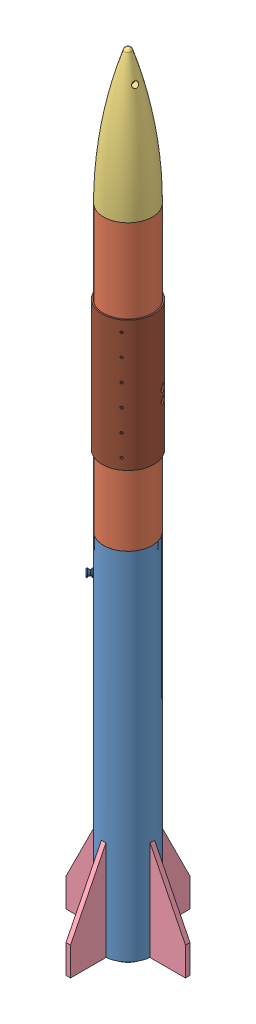
SolidWorks assembly ASSY_ROCKET_MASTER, configuration Default. Lengths in mm.
Overall size (168 1100 168).
745 component instances, 461 part files, 40 mates.
Components (placement in the parent):
- ROCKET_BODY_TUBE_LOWER-1: ROCKET_BODY_TUBE_LOWER [Default] at origin size (68.5 500 68.5)
- ROCKET_BODY_TUBE_UPPER-1: ROCKET_BODY_TUBE_UPPER [Default] at (0 500 0) x (0 0 1) z (-1 0 0) size (68.5 400 68.5)
- ROCKET_NOSE_CONE-1: ROCKET_NOSE_CONE [Default] at (0 840 0) x (0.965412 0 0.260729) z (-0.260729 0 0.965412) size (68.5 250 68.5)
- ROCKET_FIN_LOWER-1: ROCKET_FIN_LOWER [Default] at origin size (6.35 140 63)
- ROCKET_FIN_LOWER-2: ROCKET_FIN_LOWER [Default] x (0 0 1) z (-1 0 0) size (6.35 140 63)
- ROCKET_FIN_LOWER-3: ROCKET_FIN_LOWER [Default] x (-1 0 0) z (0 0 -1) size (6.35 140 63)
- ROCKET_FIN_LOWER-4: ROCKET_FIN_LOWER [Default] x (0 0 -1) z (1 0 0) size (6.35 140 63)
- ROCKET_BODY_COUPLER-1: ROCKET_BODY_COUPLER [Default] at (0 437.6 0) size (64.9 152.4 64.9)
- ASSY_HYDRA_MASTER-1: ASSY_HYDRA_MASTER [Default] at (0 713.5 0) x (0.707107 0 0.707107) z (0 1 0) size (64 66.9 228.49)
  - HYDRA_V4_NAV-1: HYDRA_V4_NAV [Default] at origin size (50 44 11.77)
    - Open CASCADE STEP translator 7.5 734-1: Open CASCADE STEP translator 7.5 734 [Default] at origin size (50 44 1.75)
    - Open CASCADE STEP translator 7.5 766-1: Open CASCADE STEP translator 7.5 766 [Default] at origin size (2.53 3.23 1.01)
    - Open CASCADE STEP translator 7.5 767-1: Open CASCADE STEP translator 7.5 767 [Default] at origin size (2.5 3.2 0)
    - Open CASCADE STEP translator 7.5 769-1: Open CASCADE STEP translator 7.5 769 [Default] at origin size (0.26 1.24 0)
    - Open CASCADE STEP translator 7.5 770-1: Open CASCADE STEP translator 7.5 770 [Default] at origin size (2.9 1.6 1.31)
    - Open CASCADE STEP translator 7.5 771-1: Open CASCADE STEP translator 7.5 771 [Default] at origin size (0.3 0.6 0.86)
    - Open CASCADE STEP translator 7.5 772-1: Open CASCADE STEP translator 7.5 772 [Default] at origin size (0.3 0.6 0.86)
    - Open CASCADE STEP translator 7.5 773-1: Open CASCADE STEP translator 7.5 773 [Default] at origin size (0.3 0.6 0.86)
    - Open CASCADE STEP translator 7.5 774-1: Open CASCADE STEP translator 7.5 774 [Default] at origin size (0.3 0.6 0.86)
    - Open CASCADE STEP translator 7.5 775-1: Open CASCADE STEP translator 7.5 775 [Default] at origin size (0.4 0.4 0.01)
    - Open CASCADE STEP translator 7.5 776-1: Open CASCADE STEP translator 7.5 776 [Default] at origin size (0.29 1.22 0.01)
    - Open CASCADE STEP translator 7.5 777-1: Open CASCADE STEP translator 7.5 777 [Default] at origin size (0.3 0.6 0.86)
    - Open CASCADE STEP translator 7.5 778-1: Open CASCADE STEP translator 7.5 778 [Default] at origin size (0.3 0.6 0.86)
    - Open CASCADE STEP translator 7.5 779-1: Open CASCADE STEP translator 7.5 779 [Default] at origin size (0.3 0.6 0.86)
    - Open CASCADE STEP translator 7.5 780-1: Open CASCADE STEP translator 7.5 780 [Default] at origin size (0.3 0.6 0.86)
    - Open CASCADE STEP translator 7.5 781-1: Open CASCADE STEP translator 7.5 781 [Default] at origin size (3.25 2.93 1.32)
    - Open CASCADE STEP translator 7.5 782-1: Open CASCADE STEP translator 7.5 782 [Default] at origin size (0.59 0.66 0.86)
    - Open CASCADE STEP translator 7.5 783-1: Open CASCADE STEP translator 7.5 783 [Default] at origin size (0.59 0.66 0.86)
    - Open CASCADE STEP translator 7.5 784-1: Open CASCADE STEP translator 7.5 784 [Default] at origin size (0.59 0.66 0.86)
    - Open CASCADE STEP translator 7.5 785-1: Open CASCADE STEP translator 7.5 785 [Default] at origin size (0.59 0.66 0.86)
    - Open CASCADE STEP translator 7.5 786-1: Open CASCADE STEP translator 7.5 786 [Default] at origin size (0.4 0.4 0.01)
    - Open CASCADE STEP translator 7.5 787-1: Open CASCADE STEP translator 7.5 787 [Default] at origin size (0.65 1.09 0.01)
    - Open CASCADE STEP translator 7.5 788-1: Open CASCADE STEP translator 7.5 788 [Default] at origin size (0.59 0.66 0.86)
    - Open CASCADE STEP translator 7.5 789-1: Open CASCADE STEP translator 7.5 789 [Default] at origin size (0.59 0.66 0.86)
    - Open CASCADE STEP translator 7.5 790-1: Open CASCADE STEP translator 7.5 790 [Default] at origin size (0.59 0.66 0.86)
    - Open CASCADE STEP translator 7.5 791-1: Open CASCADE STEP translator 7.5 791 [Default] at origin size (0.59 0.66 0.86)
    - Open CASCADE STEP translator 7.5 833-1: Open CASCADE STEP translator 7.5 833 [Default] at origin size (0.2 2.2 2.05)
    - Open CASCADE STEP translator 7.5 834-1: Open CASCADE STEP translator 7.5 834 [Default] at origin size (0.2 2.2 2.05)
    - Open CASCADE STEP translator 7.5 835-1: Open CASCADE STEP translator 7.5 835 [Default] at origin size (1.45 1.3 1.05)
    - Open CASCADE STEP translator 7.5 836-1: Open CASCADE STEP translator 7.5 836 [Default] at origin size (5.75 4.05 4.25)
    - Open CASCADE STEP translator 7.5 837-1: Open CASCADE STEP translator 7.5 837 [Default] at origin size (1.45 2.03 0.46)
    - Open CASCADE STEP translator 7.5 838-1: Open CASCADE STEP translator 7.5 838 [Default] at origin size (4.2 3.06 0.01)
    - Open CASCADE STEP translator 7.5 839-1: Open CASCADE STEP translator 7.5 839 [Default] at origin size (14.1 15.2 1.88)
    - Open CASCADE STEP translator 7.5 863-1: Open CASCADE STEP translator 7.5 863 [Default] at origin size (4.1 4.1 0.98)
    - Open CASCADE STEP translator 7.5 864-1: Open CASCADE STEP translator 7.5 864 [Default] at origin size (4.53 6.4 0.96)
    - Open CASCADE STEP translator 7.5 865-1: Open CASCADE STEP translator 7.5 865 [Default] at origin size (6.2 6.4 0.64)
    - Open CASCADE STEP translator 7.5 866-1: Open CASCADE STEP translator 7.5 866 [Default] at origin size (5.96 5.96 2.39)
    - Open CASCADE STEP translator 7.5 867-1: Open CASCADE STEP translator 7.5 867 [Default] at origin size (4.4 4.4 0.72)
    - Open CASCADE STEP translator 7.5 868-1: Open CASCADE STEP translator 7.5 868 [Default] at origin size (6.1 6 0)
    - Open CASCADE STEP translator 7.5 869-1: Open CASCADE STEP translator 7.5 869 [Default] at origin size (0.75 2.66 0)
    - Open CASCADE STEP translator 7.5 870-1: Open CASCADE STEP translator 7.5 870 [Default] at origin size (3.1 3.1 1)
    - Open CASCADE STEP translator 7.5 871-1: Open CASCADE STEP translator 7.5 871 [Default] at origin size (3 2.5 0.81)
    - Open CASCADE STEP translator 7.5 1038-1: Open CASCADE STEP translator 7.5 1038 [Default] at origin size (1.6 1.5 0.2)
    - Open CASCADE STEP translator 7.5 1039-1: Open CASCADE STEP translator 7.5 1039 [Default] at origin size (1.6 1.4 0.19)
    - Open CASCADE STEP translator 7.5 1040-1: Open CASCADE STEP translator 7.5 1040 [Default] at origin size (1.1 1.5 0.36)
    - Open CASCADE STEP translator 7.5 1113-1: Open CASCADE STEP translator 7.5 1113 [Default] at origin size (4.71 4.67 1.1)
    - Open CASCADE STEP translator 7.5 1118-1: Open CASCADE STEP translator 7.5 1118 [Default] at origin size (1.6 1.5 0.2)
    - Open CASCADE STEP translator 7.5 1119-1: Open CASCADE STEP translator 7.5 1119 [Default] at origin size (1.6 1.4 0.19)
    - Open CASCADE STEP translator 7.5 1120-1: Open CASCADE STEP translator 7.5 1120 [Default] at origin size (1.1 1.5 0.36)
    - Open CASCADE STEP translator 7.5 1124-1: Open CASCADE STEP translator 7.5 1124 [Default] at origin size (10.4 9.7 2.7)
    - Open CASCADE STEP translator 7.5 1125-1: Open CASCADE STEP translator 7.5 1125 [Default] at origin size (5 3 0.3)
    - Open CASCADE STEP translator 7.5 1126-1: Open CASCADE STEP translator 7.5 1126 [Default] at origin size (4.46 2.46 0.7)
    - Open CASCADE STEP translator 7.5 1127-1: Open CASCADE STEP translator 7.5 1127 [Default] at origin size (4.6 4.6 1.15)
    - Open CASCADE STEP translator 7.5 1128-1: Open CASCADE STEP translator 7.5 1128 [Default] at origin size (14 14 1.52)
    - Open CASCADE STEP translator 7.5 1129-1: Open CASCADE STEP translator 7.5 1129 [Default] at origin size (16 12.22 0.95)
    - Open CASCADE STEP translator 7.5 1130-1: Open CASCADE STEP translator 7.5 1130 [Default] at origin size (12.22 16 0.95)
    - Open CASCADE STEP translator 7.5 1131-1: Open CASCADE STEP translator 7.5 1131 [Default] at origin size (12.33 12.46 0.1)
    - Open CASCADE STEP translator 7.5 1132-1: Open CASCADE STEP translator 7.5 1132 [Default] at origin size (1.3 3.5 0.06)
    - Open CASCADE STEP translator 7.5 1133-1: Open CASCADE STEP translator 7.5 1133 [Default] at origin size (2 3 0.57)
    - Open CASCADE STEP translator 7.5 1134-1: Open CASCADE STEP translator 7.5 1134 [Default] at origin size (2.2 3.2 0.32)
    - Open CASCADE STEP translator 7.5 1135-1: Open CASCADE STEP translator 7.5 1135 [Default] at origin size (0.46 0.93 0.01)
    - Open CASCADE STEP translator 7.5 1136-1: Open CASCADE STEP translator 7.5 1136 [Default] at origin size (1.3 3.5 0.06)
    - Open CASCADE STEP translator 7.5 1137-1: Open CASCADE STEP translator 7.5 1137 [Default] at origin size (2 3 0.57)
    - Open CASCADE STEP translator 7.5 1138-1: Open CASCADE STEP translator 7.5 1138 [Default] at origin size (2.2 3.2 0.32)
    - Open CASCADE STEP translator 7.5 1139-1: Open CASCADE STEP translator 7.5 1139 [Default] at origin size (0.46 0.93 0.01)
    - Open CASCADE STEP translator 7.5 1209-1: Open CASCADE STEP translator 7.5 1209 [Default] at origin size (2.6 2.6 0.35)
    - Open CASCADE STEP translator 7.5 1210-1: Open CASCADE STEP translator 7.5 1210 [Default] at origin size (7.98 7.97 5.08)
    - Open CASCADE STEP translator 7.5 1211-1: Open CASCADE STEP translator 7.5 1211 [Default] at origin size (6.65 6.86 1.68)
    - Open CASCADE STEP translator 7.5 1212-1: Open CASCADE STEP translator 7.5 1212 [Default] at origin size (6.1 6.49 5.65)
    - Open CASCADE STEP translator 7.5 1213-1: Open CASCADE STEP translator 7.5 1213 [Default] at origin size (11.95 7.6 2.76)
    - Open CASCADE STEP translator 7.5 1214-1: Open CASCADE STEP translator 7.5 1214 [Default] at origin size (1.9 6.7 2.22)
    - Open CASCADE STEP translator 7.5 1215-1: Open CASCADE STEP translator 7.5 1215 [Default] at origin size (6.4 5 1.77)
    - Open CASCADE STEP translator 7.5 1216-1: Open CASCADE STEP translator 7.5 1216 [Default] at origin size (4.77 4.35 0.13)
    - Open CASCADE STEP translator 7.5 1217-1: Open CASCADE STEP translator 7.5 1217 [Default] at origin size (1.9 6.7 2.22)
    - Open CASCADE STEP translator 7.5 1293-1: Open CASCADE STEP translator 7.5 1293 [Default] at origin size (1.6 1.5 0.2)
    - Open CASCADE STEP translator 7.5 1294-1: Open CASCADE STEP translator 7.5 1294 [Default] at origin size (1.6 1.4 0.19)
    - Open CASCADE STEP translator 7.5 1295-1: Open CASCADE STEP translator 7.5 1295 [Default] at origin size (1.1 1.5 0.36)
    - Open CASCADE STEP translator 7.5 1296-1: Open CASCADE STEP translator 7.5 1296 [Default] at origin size (1.6 1.5 0.2)
    - Open CASCADE STEP translator 7.5 1297-1: Open CASCADE STEP translator 7.5 1297 [Default] at origin size (1.6 1.4 0.19)
    - Open CASCADE STEP translator 7.5 1298-1: Open CASCADE STEP translator 7.5 1298 [Default] at origin size (1.1 1.5 0.36)
    - Open CASCADE STEP translator 7.5 1299-1: Open CASCADE STEP translator 7.5 1299 [Default] at origin size (1.3 3.5 0.06)
    - Open CASCADE STEP translator 7.5 1300-1: Open CASCADE STEP translator 7.5 1300 [Default] at origin size (2 3 0.57)
    - Open CASCADE STEP translator 7.5 1301-1: Open CASCADE STEP translator 7.5 1301 [Default] at origin size (2.2 3.2 0.32)
    - Open CASCADE STEP translator 7.5 1302-1: Open CASCADE STEP translator 7.5 1302 [Default] at origin size (0.46 0.93 0.01)
    - Open CASCADE STEP translator 7.5 1303-1: Open CASCADE STEP translator 7.5 1303 [Default] at origin size (5.72 15.88 6.73)
    - Open CASCADE STEP translator 7.5 1304-1: Open CASCADE STEP translator 7.5 1304 [Default] at origin size (1.78 12.7 4.01)
    - Open CASCADE STEP translator 7.5 1305-1: Open CASCADE STEP translator 7.5 1305 [Default] at origin size (5.84 12.7 0.83)
    - Open CASCADE STEP translator 7.5 1306-1: Open CASCADE STEP translator 7.5 1306 [Default] at origin size (5.72 15.88 6.73)
    - Open CASCADE STEP translator 7.5 1307-1: Open CASCADE STEP translator 7.5 1307 [Default] at origin size (1.78 12.7 4.01)
    - Open CASCADE STEP translator 7.5 1308-1: Open CASCADE STEP translator 7.5 1308 [Default] at origin size (5.84 12.7 0.83)
    - Open CASCADE STEP translator 7.5 1309-1: Open CASCADE STEP translator 7.5 1309 [Default] at origin size (3.68 15.88 5.84)
    - Open CASCADE STEP translator 7.5 1310-1: Open CASCADE STEP translator 7.5 1310 [Default] at origin size (4.09 12.7 1.18)
    - Open CASCADE STEP translator 7.5 1311-1: Open CASCADE STEP translator 7.5 1311 [Default] at origin size (3.68 15.88 5.84)
    - Open CASCADE STEP translator 7.5 1312-1: Open CASCADE STEP translator 7.5 1312 [Default] at origin size (4.09 12.7 1.18)
  - HYDRA_V4_LINK_V2-1: HYDRA_V4_LINK_V2 [Default] at (-0.0024 -0.0016 7.6116) size (50 44 11.77)
    - Open CASCADE STEP translator 7.5 1-1: Open CASCADE STEP translator 7.5 1 [Default] at origin size (50 44 1.61)
    - Open CASCADE STEP translator 7.5 16-1: Open CASCADE STEP translator 7.5 16 [Default] at origin size (13.25 4.05 4.25)
    - Open CASCADE STEP translator 7.5 17-1: Open CASCADE STEP translator 7.5 17 [Default] at origin size (0.2 4.65 2.09)
    - Open CASCADE STEP translator 7.5 18-1: Open CASCADE STEP translator 7.5 18 [Default] at origin size (0.2 4.65 2.09)
    - Open CASCADE STEP translator 7.5 19-1: Open CASCADE STEP translator 7.5 19 [Default] at origin size (0.2 4.65 2.09)
    - Open CASCADE STEP translator 7.5 20-1: Open CASCADE STEP translator 7.5 20 [Default] at origin size (0.2 4.65 2.09)
    - Open CASCADE STEP translator 7.5 21-1: Open CASCADE STEP translator 7.5 21 [Default] at origin size (0.2 4.65 2.09)
    - Open CASCADE STEP translator 7.5 22-1: Open CASCADE STEP translator 7.5 22 [Default] at origin size (0.2 4.65 2.09)
    - Open CASCADE STEP translator 7.5 23-1: Open CASCADE STEP translator 7.5 23 [Default] at origin size (0.2 4.65 2.09)
    - Open CASCADE STEP translator 7.5 24-1: Open CASCADE STEP translator 7.5 24 [Default] at origin size (0.2 4.65 2.09)
    - Open CASCADE STEP translator 7.5 86-1: Open CASCADE STEP translator 7.5 86 [Default] at origin size (2.15 1.35 0.85)
    - Open CASCADE STEP translator 7.5 87-1: Open CASCADE STEP translator 7.5 87 [Default] at origin size (2.15 1.35 0.85)
    - Open CASCADE STEP translator 7.5 88-1: Open CASCADE STEP translator 7.5 88 [Default] at origin size (1.21 0.73 0.02)
    - Open CASCADE STEP translator 7.5 89-1: Open CASCADE STEP translator 7.5 89 [Default] at origin size (3.23 2.53 1.01)
    - Open CASCADE STEP translator 7.5 90-1: Open CASCADE STEP translator 7.5 90 [Default] at origin size (3.2 2.5 0)
    - Open CASCADE STEP translator 7.5 91-1: Open CASCADE STEP translator 7.5 91 [Default] at origin size (0.25 0.25 0.01)
    - Open CASCADE STEP translator 7.5 92-1: Open CASCADE STEP translator 7.5 92 [Default] at origin size (1.24 0.26 0)
    - Open CASCADE STEP translator 7.5 93-1: Open CASCADE STEP translator 7.5 93 [Default] at origin size (3.25 2.93 1.32)
    - Open CASCADE STEP translator 7.5 94-1: Open CASCADE STEP translator 7.5 94 [Default] at origin size (0.59 0.66 0.86)
    - Open CASCADE STEP translator 7.5 95-1: Open CASCADE STEP translator 7.5 95 [Default] at origin size (0.59 0.66 0.86)
    - Open CASCADE STEP translator 7.5 96-1: Open CASCADE STEP translator 7.5 96 [Default] at origin size (0.59 0.66 0.86)
    - Open CASCADE STEP translator 7.5 97-1: Open CASCADE STEP translator 7.5 97 [Default] at origin size (0.59 0.66 0.86)
    - Open CASCADE STEP translator 7.5 98-1: Open CASCADE STEP translator 7.5 98 [Default] at origin size (0.4 0.4 0.01)
    - Open CASCADE STEP translator 7.5 99-1: Open CASCADE STEP translator 7.5 99 [Default] at origin size (0.65 1.09 0.01)
    - Open CASCADE STEP translator 7.5 100-1: Open CASCADE STEP translator 7.5 100 [Default] at origin size (0.59 0.66 0.86)
    - Open CASCADE STEP translator 7.5 101-1: Open CASCADE STEP translator 7.5 101 [Default] at origin size (0.59 0.66 0.86)
    - Open CASCADE STEP translator 7.5 102-1: Open CASCADE STEP translator 7.5 102 [Default] at origin size (0.59 0.66 0.86)
    - Open CASCADE STEP translator 7.5 103-1: Open CASCADE STEP translator 7.5 103 [Default] at origin size (0.59 0.66 0.86)
    - Open CASCADE STEP translator 7.5 104-1: Open CASCADE STEP translator 7.5 104 [Default] at origin size (4.71 4.67 1.1)
    - Open CASCADE STEP translator 7.5 105-1: Open CASCADE STEP translator 7.5 105 [Default] at origin size (11.99 11.99 1.61)
    - Open CASCADE STEP translator 7.5 106-1: Open CASCADE STEP translator 7.5 106 [Default] at origin size (1.3 3.5 0.06)
    - Open CASCADE STEP translator 7.5 107-1: Open CASCADE STEP translator 7.5 107 [Default] at origin size (2 3 0.57)
    - Open CASCADE STEP translator 7.5 108-1: Open CASCADE STEP translator 7.5 108 [Default] at origin size (2.2 3.2 0.32)
    - Open CASCADE STEP translator 7.5 109-1: Open CASCADE STEP translator 7.5 109 [Default] at origin size (0.46 0.93 0.01)
    - Open CASCADE STEP translator 7.5 157-1: Open CASCADE STEP translator 7.5 157 [Default] at origin size (3.23 2.53 1.01)
    - Open CASCADE STEP translator 7.5 158-1: Open CASCADE STEP translator 7.5 158 [Default] at origin size (3.2 2.5 0)
    - Open CASCADE STEP translator 7.5 159-1: Open CASCADE STEP translator 7.5 159 [Default] at origin size (0.25 0.25 0.01)
    - Open CASCADE STEP translator 7.5 160-1: Open CASCADE STEP translator 7.5 160 [Default] at origin size (1.24 0.26 0)
    - Open CASCADE STEP translator 7.5 161-1: Open CASCADE STEP translator 7.5 161 [Default] at origin size (0.88 0.88 0)
    - Open CASCADE STEP translator 7.5 162-1: Open CASCADE STEP translator 7.5 162 [Default] at origin size (7.01 7.01 1.57)
    - Open CASCADE STEP translator 7.5 163-1: Open CASCADE STEP translator 7.5 163 [Default] at origin size (0.22 1 0.88)
    - Open CASCADE STEP translator 7.5 164-1: Open CASCADE STEP translator 7.5 164 [Default] at origin size (0.22 1 0.88)
    - Open CASCADE STEP translator 7.5 165-1: Open CASCADE STEP translator 7.5 165 [Default] at origin size (0.22 1 0.88)
    - Open CASCADE STEP translator 7.5 166-1: Open CASCADE STEP translator 7.5 166 [Default] at origin size (0.22 1 0.88)
    - Open CASCADE STEP translator 7.5 167-1: Open CASCADE STEP translator 7.5 167 [Default] at origin size (0.22 1 0.88)
    - Open CASCADE STEP translator 7.5 168-1: Open CASCADE STEP translator 7.5 168 [Default] at origin size (0.22 1 0.88)
    - Open CASCADE STEP translator 7.5 169-1: Open CASCADE STEP translator 7.5 169 [Default] at origin size (0.22 1 0.88)
    - Open CASCADE STEP translator 7.5 170-1: Open CASCADE STEP translator 7.5 170 [Default] at origin size (0.22 1 0.88)
    - Open CASCADE STEP translator 7.5 171-1: Open CASCADE STEP translator 7.5 171 [Default] at origin size (0.22 1 0.88)
    - Open CASCADE STEP translator 7.5 172-1: Open CASCADE STEP translator 7.5 172 [Default] at origin size (0.22 1 0.88)
    - Open CASCADE STEP translator 7.5 173-1: Open CASCADE STEP translator 7.5 173 [Default] at origin size (0.22 1 0.88)
    - Open CASCADE STEP translator 7.5 174-1: Open CASCADE STEP translator 7.5 174 [Default] at origin size (0.22 1 0.88)
    - Open CASCADE STEP translator 7.5 175-1: Open CASCADE STEP translator 7.5 175 [Default] at origin size (0.22 1 0.88)
    - Open CASCADE STEP translator 7.5 176-1: Open CASCADE STEP translator 7.5 176 [Default] at origin size (0.22 1 0.88)
    - Open CASCADE STEP translator 7.5 177-1: Open CASCADE STEP translator 7.5 177 [Default] at origin size (0.22 1 0.88)
    - Open CASCADE STEP translator 7.5 178-1: Open CASCADE STEP translator 7.5 178 [Default] at origin size (0.22 1 0.88)
    - Open CASCADE STEP translator 7.5 179-1: Open CASCADE STEP translator 7.5 179 [Default] at origin size (0.22 1 0.88)
    - Open CASCADE STEP translator 7.5 180-1: Open CASCADE STEP translator 7.5 180 [Default] at origin size (0.22 1 0.88)
    - Open CASCADE STEP translator 7.5 181-1: Open CASCADE STEP translator 7.5 181 [Default] at origin size (0.22 1 0.88)
    - Open CASCADE STEP translator 7.5 182-1: Open CASCADE STEP translator 7.5 182 [Default] at origin size (0.22 1 0.88)
    - Open CASCADE STEP translator 7.5 183-1: Open CASCADE STEP translator 7.5 183 [Default] at origin size (0.22 1 0.88)
    - Open CASCADE STEP translator 7.5 184-1: Open CASCADE STEP translator 7.5 184 [Default] at origin size (0.22 1 0.88)
    - Open CASCADE STEP translator 7.5 185-1: Open CASCADE STEP translator 7.5 185 [Default] at origin size (0.22 1 0.88)
    - Open CASCADE STEP translator 7.5 186-1: Open CASCADE STEP translator 7.5 186 [Default] at origin size (0.22 1 0.88)
    - Open CASCADE STEP translator 7.5 187-1: Open CASCADE STEP translator 7.5 187 [Default] at origin size (1 0.22 0.88)
    - Open CASCADE STEP translator 7.5 188-1: Open CASCADE STEP translator 7.5 188 [Default] at origin size (1 0.22 0.88)
    - Open CASCADE STEP translator 7.5 189-1: Open CASCADE STEP translator 7.5 189 [Default] at origin size (1 0.22 0.88)
    - Open CASCADE STEP translator 7.5 190-1: Open CASCADE STEP translator 7.5 190 [Default] at origin size (1 0.22 0.88)
    - Open CASCADE STEP translator 7.5 191-1: Open CASCADE STEP translator 7.5 191 [Default] at origin size (1 0.22 0.88)
    - Open CASCADE STEP translator 7.5 192-1: Open CASCADE STEP translator 7.5 192 [Default] at origin size (1 0.22 0.88)
    - Open CASCADE STEP translator 7.5 193-1: Open CASCADE STEP translator 7.5 193 [Default] at origin size (1 0.22 0.88)
    - Open CASCADE STEP translator 7.5 194-1: Open CASCADE STEP translator 7.5 194 [Default] at origin size (1 0.22 0.88)
    - Open CASCADE STEP translator 7.5 195-1: Open CASCADE STEP translator 7.5 195 [Default] at origin size (1 0.22 0.88)
    - Open CASCADE STEP translator 7.5 196-1: Open CASCADE STEP translator 7.5 196 [Default] at origin size (1 0.22 0.88)
    - Open CASCADE STEP translator 7.5 197-1: Open CASCADE STEP translator 7.5 197 [Default] at origin size (1 0.22 0.88)
    - Open CASCADE STEP translator 7.5 198-1: Open CASCADE STEP translator 7.5 198 [Default] at origin size (1 0.22 0.88)
    - Open CASCADE STEP translator 7.5 199-1: Open CASCADE STEP translator 7.5 199 [Default] at origin size (1 0.22 0.88)
    - Open CASCADE STEP translator 7.5 200-1: Open CASCADE STEP translator 7.5 200 [Default] at origin size (1 0.22 0.88)
    - Open CASCADE STEP translator 7.5 201-1: Open CASCADE STEP translator 7.5 201 [Default] at origin size (1 0.22 0.88)
    - Open CASCADE STEP translator 7.5 202-1: Open CASCADE STEP translator 7.5 202 [Default] at origin size (1 0.22 0.88)
    - Open CASCADE STEP translator 7.5 203-1: Open CASCADE STEP translator 7.5 203 [Default] at origin size (1 0.22 0.88)
    - Open CASCADE STEP translator 7.5 204-1: Open CASCADE STEP translator 7.5 204 [Default] at origin size (1 0.22 0.88)
    - Open CASCADE STEP translator 7.5 205-1: Open CASCADE STEP translator 7.5 205 [Default] at origin size (1 0.22 0.88)
    - Open CASCADE STEP translator 7.5 206-1: Open CASCADE STEP translator 7.5 206 [Default] at origin size (1 0.22 0.88)
    - Open CASCADE STEP translator 7.5 207-1: Open CASCADE STEP translator 7.5 207 [Default] at origin size (1 0.22 0.88)
    - Open CASCADE STEP translator 7.5 208-1: Open CASCADE STEP translator 7.5 208 [Default] at origin size (1 0.22 0.88)
    - Open CASCADE STEP translator 7.5 209-1: Open CASCADE STEP translator 7.5 209 [Default] at origin size (1 0.22 0.88)
    - Open CASCADE STEP translator 7.5 210-1: Open CASCADE STEP translator 7.5 210 [Default] at origin size (1 0.22 0.88)
    - Open CASCADE STEP translator 7.5 212-1: Open CASCADE STEP translator 7.5 212 [Default] at origin size (3 3 1)
    - Open CASCADE STEP translator 7.5 213-1: Open CASCADE STEP translator 7.5 213 [Default] at origin size (3 3 0.8)
    - Open CASCADE STEP translator 7.5 215-1: Open CASCADE STEP translator 7.5 215 [Default] at origin size (4 3 0.2)
    - Open CASCADE STEP translator 7.5 216-1: Open CASCADE STEP translator 7.5 216 [Default] at origin size (4.02 3.02 0.99)
    - Open CASCADE STEP translator 7.5 217-1: Open CASCADE STEP translator 7.5 217 [Default] at origin size (0.36 1.52 0.02)
    - Open CASCADE STEP translator 7.5 218-1: Open CASCADE STEP translator 7.5 218 [Default] at origin size (0.3 0.3 0.01)
    - Open CASCADE STEP translator 7.5 219-1: Open CASCADE STEP translator 7.5 219 [Default] at origin size (3 3 0.8)
    - Open CASCADE STEP translator 7.5 220-1: Open CASCADE STEP translator 7.5 220 [Default] at origin size (2 2 0.8)
    - Open CASCADE STEP translator 7.5 221-1: Open CASCADE STEP translator 7.5 221 [Default] at origin size (3.1 3.1 1)
    - Open CASCADE STEP translator 7.5 222-1: Open CASCADE STEP translator 7.5 222 [Default] at origin size (3.1 3.1 1)
    - Open CASCADE STEP translator 7.5 223-1: Open CASCADE STEP translator 7.5 223 [Default] at origin size (12.71 9.54 2.17)
    - Open CASCADE STEP translator 7.5 509-1: Open CASCADE STEP translator 7.5 509 [Default] at origin size (4.07 4.06 1.2)
    - Open CASCADE STEP translator 7.5 510-1: Open CASCADE STEP translator 7.5 510 [Default] at origin size (2 4.45 0.9)
    - Open CASCADE STEP translator 7.5 511-1: Open CASCADE STEP translator 7.5 511 [Default] at origin size (1.26 1.48 0.01)
    - Open CASCADE STEP translator 7.5 512-1: Open CASCADE STEP translator 7.5 512 [Default] at origin size (3.99 3.99 0.1)
    - Open CASCADE STEP translator 7.5 513-1: Open CASCADE STEP translator 7.5 513 [Default] at origin size (4.06 4.07 1.2)
    - Open CASCADE STEP translator 7.5 514-1: Open CASCADE STEP translator 7.5 514 [Default] at origin size (4.45 2 0.9)
    - Open CASCADE STEP translator 7.5 515-1: Open CASCADE STEP translator 7.5 515 [Default] at origin size (1.48 1.26 0.01)
    - Open CASCADE STEP translator 7.5 516-1: Open CASCADE STEP translator 7.5 516 [Default] at origin size (3.99 3.99 0.1)
    - Open CASCADE STEP translator 7.5 529-1: Open CASCADE STEP translator 7.5 529 [Default] at origin size (1.6 1.5 0.2)
    - Open CASCADE STEP translator 7.5 530-1: Open CASCADE STEP translator 7.5 530 [Default] at origin size (1.6 1.4 0.19)
    - Open CASCADE STEP translator 7.5 531-1: Open CASCADE STEP translator 7.5 531 [Default] at origin size (1.1 1.5 0.36)
    - Open CASCADE STEP translator 7.5 532-1: Open CASCADE STEP translator 7.5 532 [Default] at origin size (1.6 1.5 0.2)
    - Open CASCADE STEP translator 7.5 533-1: Open CASCADE STEP translator 7.5 533 [Default] at origin size (1.6 1.4 0.19)
    - Open CASCADE STEP translator 7.5 534-1: Open CASCADE STEP translator 7.5 534 [Default] at origin size (1.1 1.5 0.36)
    - Open CASCADE STEP translator 7.5 626-1: Open CASCADE STEP translator 7.5 626 [Default] at origin size (2.8 3.3 2)
    - Open CASCADE STEP translator 7.5 627-1: Open CASCADE STEP translator 7.5 627 [Default] at origin size (2.2 0.8 1)
    - Open CASCADE STEP translator 7.5 628-1: Open CASCADE STEP translator 7.5 628 [Default] at origin size (2.2 0.8 1)
    - Open CASCADE STEP translator 7.5 629-1: Open CASCADE STEP translator 7.5 629 [Default] at origin size (2.11 2.66 0.01)
    - Open CASCADE STEP translator 7.5 636-1: Open CASCADE STEP translator 7.5 636 [Default] at origin size (2.01 1.26 1.46)
    - Open CASCADE STEP translator 7.5 637-1: Open CASCADE STEP translator 7.5 637 [Default] at origin size (1 1.25 1.45)
    - Open CASCADE STEP translator 7.5 638-1: Open CASCADE STEP translator 7.5 638 [Default] at origin size (0.67 0.05 0.01)
    - Open CASCADE STEP translator 7.5 639-1: Open CASCADE STEP translator 7.5 639 [Default] at origin size (1.1 1.25 1.45)
    - Open CASCADE STEP translator 7.5 640-1: Open CASCADE STEP translator 7.5 640 [Default] at origin size (0.46 1.26 1.46)
    - Open CASCADE STEP translator 7.5 641-1: Open CASCADE STEP translator 7.5 641 [Default] at origin size (0.46 1.26 1.46)
    - Open CASCADE STEP translator 7.5 642-1: Open CASCADE STEP translator 7.5 642 [Default] at origin size (0.61 0.15 0.01)
    - Open CASCADE STEP translator 7.5 643-1: Open CASCADE STEP translator 7.5 643 [Default] at origin size (1.1 1.25 1.45)
    - Open CASCADE STEP translator 7.5 644-1: Open CASCADE STEP translator 7.5 644 [Default] at origin size (0.46 1.26 1.46)
    - Open CASCADE STEP translator 7.5 645-1: Open CASCADE STEP translator 7.5 645 [Default] at origin size (0.46 1.26 1.46)
    - Open CASCADE STEP translator 7.5 646-1: Open CASCADE STEP translator 7.5 646 [Default] at origin size (0.61 0.15 0.01)
    - Open CASCADE STEP translator 7.5 662-1: Open CASCADE STEP translator 7.5 662 [Default] at origin size (3.3 2.8 2)
    - Open CASCADE STEP translator 7.5 663-1: Open CASCADE STEP translator 7.5 663 [Default] at origin size (0.8 2.2 1)
    - Open CASCADE STEP translator 7.5 664-1: Open CASCADE STEP translator 7.5 664 [Default] at origin size (0.8 2.2 1)
    - Open CASCADE STEP translator 7.5 665-1: Open CASCADE STEP translator 7.5 665 [Default] at origin size (2.66 2.11 0.01)
    - Open CASCADE STEP translator 7.5 669-1: Open CASCADE STEP translator 7.5 669 [Default] at origin size (1.27 2.02 1.42)
    - Open CASCADE STEP translator 7.5 670-1: Open CASCADE STEP translator 7.5 670 [Default] at origin size (1.25 2 1.4)
    - Open CASCADE STEP translator 7.5 671-1: Open CASCADE STEP translator 7.5 671 [Default] at origin size (0.12 0.53 0.1)
    - Open CASCADE STEP translator 7.5 672-1: Open CASCADE STEP translator 7.5 672 [Default] at origin size (1.27 2.02 1.42)
    - Open CASCADE STEP translator 7.5 673-1: Open CASCADE STEP translator 7.5 673 [Default] at origin size (1.25 2 1.4)
    - Open CASCADE STEP translator 7.5 674-1: Open CASCADE STEP translator 7.5 674 [Default] at origin size (0.12 0.53 0.1)
    - Open CASCADE STEP translator 7.5 675-1: Open CASCADE STEP translator 7.5 675 [Default] at origin size (1.27 2.02 1.42)
    - Open CASCADE STEP translator 7.5 676-1: Open CASCADE STEP translator 7.5 676 [Default] at origin size (1.25 2 1.4)
    - Open CASCADE STEP translator 7.5 677-1: Open CASCADE STEP translator 7.5 677 [Default] at origin size (0.12 0.53 0.1)
    - Open CASCADE STEP translator 7.5 678-1: Open CASCADE STEP translator 7.5 678 [Default] at origin size (1.25 0.5 1.4)
    - Open CASCADE STEP translator 7.5 679-1: Open CASCADE STEP translator 7.5 679 [Default] at origin size (1.25 0.5 1.4)
    - Open CASCADE STEP translator 7.5 680-1: Open CASCADE STEP translator 7.5 680 [Default] at origin size (1.15 1 1.3)
    - Open CASCADE STEP translator 7.5 681-1: Open CASCADE STEP translator 7.5 681 [Default] at origin size (1.25 0.5 1.4)
    - Open CASCADE STEP translator 7.5 682-1: Open CASCADE STEP translator 7.5 682 [Default] at origin size (1.25 0.5 1.4)
    - Open CASCADE STEP translator 7.5 683-1: Open CASCADE STEP translator 7.5 683 [Default] at origin size (1.15 1 1.3)
    - Open CASCADE STEP translator 7.5 687-1: Open CASCADE STEP translator 7.5 687 [Default] at origin size (0.5 1.25 1.4)
    - Open CASCADE STEP translator 7.5 688-1: Open CASCADE STEP translator 7.5 688 [Default] at origin size (0.5 1.25 1.4)
    - Open CASCADE STEP translator 7.5 689-1: Open CASCADE STEP translator 7.5 689 [Default] at origin size (1 1.15 1.3)
    - Open CASCADE STEP translator 7.5 708-1: Open CASCADE STEP translator 7.5 708 [Default] at origin size (1.6 1.5 0.2)
    - Open CASCADE STEP translator 7.5 709-1: Open CASCADE STEP translator 7.5 709 [Default] at origin size (1.6 1.4 0.19)
    - Open CASCADE STEP translator 7.5 710-1: Open CASCADE STEP translator 7.5 710 [Default] at origin size (1.1 1.5 0.36)
    - Open CASCADE STEP translator 7.5 711-1: Open CASCADE STEP translator 7.5 711 [Default] at origin size (1.6 1.5 0.2)
    - Open CASCADE STEP translator 7.5 712-1: Open CASCADE STEP translator 7.5 712 [Default] at origin size (1.6 1.4 0.19)
    - Open CASCADE STEP translator 7.5 713-1: Open CASCADE STEP translator 7.5 713 [Default] at origin size (1.1 1.5 0.36)
    - Open CASCADE STEP translator 7.5 714-1: Open CASCADE STEP translator 7.5 714 [Default] at origin size (17 16 3.32)
    - Open CASCADE STEP translator 7.5 715-1: Open CASCADE STEP translator 7.5 715 [Default] at origin size (3.68 15.88 5.84)
    - Open CASCADE STEP translator 7.5 716-1: Open CASCADE STEP translator 7.5 716 [Default] at origin size (4.09 12.7 1.18)
    - Open CASCADE STEP translator 7.5 717-1: Open CASCADE STEP translator 7.5 717 [Default] at origin size (3.68 15.88 5.84)
    - Open CASCADE STEP translator 7.5 718-1: Open CASCADE STEP translator 7.5 718 [Default] at origin size (4.09 12.7 1.18)
    - Open CASCADE STEP translator 7.5 719-1: Open CASCADE STEP translator 7.5 719 [Default] at origin size (1.3 3.5 0.06)
    - Open CASCADE STEP translator 7.5 720-1: Open CASCADE STEP translator 7.5 720 [Default] at origin size (2 3 0.57)
    - Open CASCADE STEP translator 7.5 721-1: Open CASCADE STEP translator 7.5 721 [Default] at origin size (2.2 3.2 0.32)
    - Open CASCADE STEP translator 7.5 722-1: Open CASCADE STEP translator 7.5 722 [Default] at origin size (0.46 0.93 0.01)
    - Open CASCADE STEP translator 7.5 723-1: Open CASCADE STEP translator 7.5 723 [Default] at origin size (14.1 15.2 1.88)
    - Open CASCADE STEP translator 7.5 725-1: Open CASCADE STEP translator 7.5 725 [Default] at origin size (7.98 7.97 5.08)
    - Open CASCADE STEP translator 7.5 726-1: Open CASCADE STEP translator 7.5 726 [Default] at origin size (6.65 6.86 1.68)
    - Open CASCADE STEP translator 7.5 727-1: Open CASCADE STEP translator 7.5 727 [Default] at origin size (6.1 6.49 5.65)
    - Open CASCADE STEP translator 7.5 728-1: Open CASCADE STEP translator 7.5 728 [Default] at origin size (5.72 15.88 6.73)
    - Open CASCADE STEP translator 7.5 729-1: Open CASCADE STEP translator 7.5 729 [Default] at origin size (1.78 12.7 4.01)
    - Open CASCADE STEP translator 7.5 730-1: Open CASCADE STEP translator 7.5 730 [Default] at origin size (5.84 12.7 0.83)
    - Open CASCADE STEP translator 7.5 731-1: Open CASCADE STEP translator 7.5 731 [Default] at origin size (5.72 15.88 6.73)
    - Open CASCADE STEP translator 7.5 732-1: Open CASCADE STEP translator 7.5 732 [Default] at origin size (1.78 12.7 4.01)
    - Open CASCADE STEP translator 7.5 733-1: Open CASCADE STEP translator 7.5 733 [Default] at origin size (5.84 12.7 0.83)
  - HYDRA_V4_RECOVERY-1: HYDRA_V4_RECOVERY [Default] at (-0.0049 -0.0019 15.2232) size (50.1 44.1 11.77)
    - Open CASCADE STEP translator 7.5 2755-1: Open CASCADE STEP translator 7.5 2755 [Default] at origin size (50.1 44.1 1.61)
    - Open CASCADE STEP translator 7.5 2760-1: Open CASCADE STEP translator 7.5 2760 [Default] at origin size (3.1 3.1 1)
    - Open CASCADE STEP translator 7.5 2790-1: Open CASCADE STEP translator 7.5 2790 [Default] at origin size (14.6 14.5 1.9)
    - Open CASCADE STEP translator 7.5 2825-1: Open CASCADE STEP translator 7.5 2825 [Default] at origin size (1.3 3.5 0.06)
    - Open CASCADE STEP translator 7.5 2826-1: Open CASCADE STEP translator 7.5 2826 [Default] at origin size (2 3 0.57)
    - Open CASCADE STEP translator 7.5 2827-1: Open CASCADE STEP translator 7.5 2827 [Default] at origin size (2.2 3.2 0.32)
    - Open CASCADE STEP translator 7.5 2828-1: Open CASCADE STEP translator 7.5 2828 [Default] at origin size (0.46 0.93 0.01)
    - Open CASCADE STEP translator 7.5 2844-1: Open CASCADE STEP translator 7.5 2844 [Default] at origin size (2.53 3.23 1.01)
    - Open CASCADE STEP translator 7.5 2845-1: Open CASCADE STEP translator 7.5 2845 [Default] at origin size (2.5 3.2 0)
    - Open CASCADE STEP translator 7.5 2846-1: Open CASCADE STEP translator 7.5 2846 [Default] at origin size (0.25 0.25 0.01)
    - Open CASCADE STEP translator 7.5 2847-1: Open CASCADE STEP translator 7.5 2847 [Default] at origin size (0.26 1.24 0)
    - Open CASCADE STEP translator 7.5 2848-1: Open CASCADE STEP translator 7.5 2848 [Default] at origin size (3.62 3.76 1.01)
    - Open CASCADE STEP translator 7.5 2849-1: Open CASCADE STEP translator 7.5 2849 [Default] at origin size (3.62 3.76 0)
    - Open CASCADE STEP translator 7.5 2851-1: Open CASCADE STEP translator 7.5 2851 [Default] at origin size (0.81 1.11 0)
    - Open CASCADE STEP translator 7.5 2852-1: Open CASCADE STEP translator 7.5 2852 [Default] at origin size (4.71 4.67 1.1)
    - Open CASCADE STEP translator 7.5 2853-1: Open CASCADE STEP translator 7.5 2853 [Default] at origin size (3.25 2.93 1.32)
    - Open CASCADE STEP translator 7.5 2854-1: Open CASCADE STEP translator 7.5 2854 [Default] at origin size (0.59 0.66 0.86)
    - Open CASCADE STEP translator 7.5 2855-1: Open CASCADE STEP translator 7.5 2855 [Default] at origin size (0.59 0.66 0.86)
    - Open CASCADE STEP translator 7.5 2856-1: Open CASCADE STEP translator 7.5 2856 [Default] at origin size (0.59 0.66 0.86)
    - Open CASCADE STEP translator 7.5 2857-1: Open CASCADE STEP translator 7.5 2857 [Default] at origin size (0.59 0.66 0.86)
    - Open CASCADE STEP translator 7.5 2858-1: Open CASCADE STEP translator 7.5 2858 [Default] at origin size (0.4 0.4 0.01)
    - Open CASCADE STEP translator 7.5 2859-1: Open CASCADE STEP translator 7.5 2859 [Default] at origin size (0.65 1.09 0.01)
    - Open CASCADE STEP translator 7.5 2860-1: Open CASCADE STEP translator 7.5 2860 [Default] at origin size (0.59 0.66 0.86)
    - Open CASCADE STEP translator 7.5 2861-1: Open CASCADE STEP translator 7.5 2861 [Default] at origin size (0.59 0.66 0.86)
    - Open CASCADE STEP translator 7.5 2862-1: Open CASCADE STEP translator 7.5 2862 [Default] at origin size (0.59 0.66 0.86)
    - Open CASCADE STEP translator 7.5 2863-1: Open CASCADE STEP translator 7.5 2863 [Default] at origin size (0.59 0.66 0.86)
    - Open CASCADE STEP translator 7.5 2864-1: Open CASCADE STEP translator 7.5 2864 [Default] at origin size (14 14 1.52)
    - Open CASCADE STEP translator 7.5 2865-1: Open CASCADE STEP translator 7.5 2865 [Default] at origin size (16 12.22 0.95)
    - Open CASCADE STEP translator 7.5 2866-1: Open CASCADE STEP translator 7.5 2866 [Default] at origin size (12.22 16 0.95)
    - Open CASCADE STEP translator 7.5 2867-1: Open CASCADE STEP translator 7.5 2867 [Default] at origin size (12.33 12.46 0.1)
    - Open CASCADE STEP translator 7.5 2868-1: Open CASCADE STEP translator 7.5 2868 [Default] at origin size (5.02 5.02 0.79)
    - Open CASCADE STEP translator 7.5 2869-1: Open CASCADE STEP translator 7.5 2869 [Default] at origin size (5 5 0.2)
    - Open CASCADE STEP translator 7.5 2870-1: Open CASCADE STEP translator 7.5 2870 [Default] at origin size (0.51 0.51 0.01)
    - Open CASCADE STEP translator 7.5 2871-1: Open CASCADE STEP translator 7.5 2871 [Default] at origin size (2.27 0.67 0.03)
    - Open CASCADE STEP translator 7.5 2873-1: Open CASCADE STEP translator 7.5 2873 [Default] at origin size (5 3 0.3)
    - Open CASCADE STEP translator 7.5 2874-1: Open CASCADE STEP translator 7.5 2874 [Default] at origin size (4.46 2.46 0.7)
    - Open CASCADE STEP translator 7.5 2875-1: Open CASCADE STEP translator 7.5 2875 [Default] at origin size (4.6 4.6 1.15)
    - Open CASCADE STEP translator 7.5 2876-1: Open CASCADE STEP translator 7.5 2876 [Default] at origin size (3.1 3.1 1)
    - Open CASCADE STEP translator 7.5 2877-1: Open CASCADE STEP translator 7.5 2877 [Default] at origin size (3 3 0.8)
    - Open CASCADE STEP translator 7.5 2878-1: Open CASCADE STEP translator 7.5 2878 [Default] at origin size (3 3 0.8)
    - Open CASCADE STEP translator 7.5 3138-1: Open CASCADE STEP translator 7.5 3138 [Default] at origin size (3 3 0.86)
    - Open CASCADE STEP translator 7.5 3139-1: Open CASCADE STEP translator 7.5 3139 [Default] at origin size (3.2 3.1 0.15)
    - Open CASCADE STEP translator 7.5 3140-1: Open CASCADE STEP translator 7.5 3140 [Default] at origin size (0.53 2.36 0.02)
    - Open CASCADE STEP translator 7.5 3141-1: Open CASCADE STEP translator 7.5 3141 [Default] at origin size (3 3 0.86)
    - Open CASCADE STEP translator 7.5 3142-1: Open CASCADE STEP translator 7.5 3142 [Default] at origin size (3.2 3.1 0.15)
    - Open CASCADE STEP translator 7.5 3143-1: Open CASCADE STEP translator 7.5 3143 [Default] at origin size (0.53 2.36 0.02)
    - Open CASCADE STEP translator 7.5 3148-1: Open CASCADE STEP translator 7.5 3148 [Default] at origin size (3 3 0.86)
    - Open CASCADE STEP translator 7.5 3149-1: Open CASCADE STEP translator 7.5 3149 [Default] at origin size (3.1 3.2 0.15)
    - Open CASCADE STEP translator 7.5 3150-1: Open CASCADE STEP translator 7.5 3150 [Default] at origin size (2.36 0.53 0.02)
    - Open CASCADE STEP translator 7.5 3160-1: Open CASCADE STEP translator 7.5 3160 [Default] at origin size (3 3 0.86)
    - Open CASCADE STEP translator 7.5 3161-1: Open CASCADE STEP translator 7.5 3161 [Default] at origin size (3.1 3.2 0.15)
    - Open CASCADE STEP translator 7.5 3162-1: Open CASCADE STEP translator 7.5 3162 [Default] at origin size (2.36 0.53 0.02)
    - Open CASCADE STEP translator 7.5 3163-1: Open CASCADE STEP translator 7.5 3163 [Default] at origin size (8.53 8.53 4)
    - Open CASCADE STEP translator 7.5 3164-1: Open CASCADE STEP translator 7.5 3164 [Default] at origin size (0.2 2.2 2.05)
    - Open CASCADE STEP translator 7.5 3165-1: Open CASCADE STEP translator 7.5 3165 [Default] at origin size (0.2 2.2 2.05)
    - Open CASCADE STEP translator 7.5 3166-1: Open CASCADE STEP translator 7.5 3166 [Default] at origin size (1.45 1.3 1.05)
    - Open CASCADE STEP translator 7.5 3167-1: Open CASCADE STEP translator 7.5 3167 [Default] at origin size (5.75 4.05 4.25)
    - Open CASCADE STEP translator 7.5 3168-1: Open CASCADE STEP translator 7.5 3168 [Default] at origin size (1.45 2.03 0.46)
    - Open CASCADE STEP translator 7.5 3169-1: Open CASCADE STEP translator 7.5 3169 [Default] at origin size (4.2 3.06 0.01)
    - Open CASCADE STEP translator 7.5 3170-1: Open CASCADE STEP translator 7.5 3170 [Default] at origin size (6.45 4.3 2.13)
    - Open CASCADE STEP translator 7.5 3171-1: Open CASCADE STEP translator 7.5 3171 [Default] at origin size (10.75 4.05 4.35)
    - Open CASCADE STEP translator 7.5 3172-1: Open CASCADE STEP translator 7.5 3172 [Default] at origin size (10.15 2.2 3)
    - Open CASCADE STEP translator 7.5 3174-1: Open CASCADE STEP translator 7.5 3174 [Default] at origin size (6.45 4.3 2.13)
    - Open CASCADE STEP translator 7.5 3175-1: Open CASCADE STEP translator 7.5 3175 [Default] at origin size (10.75 4.05 4.35)
    - Open CASCADE STEP translator 7.5 3176-1: Open CASCADE STEP translator 7.5 3176 [Default] at origin size (10.15 2.2 3)
    - Open CASCADE STEP translator 7.5 3177-1: Open CASCADE STEP translator 7.5 3177 [Default] at origin size (0.46 0.01 0.54)
    - Open CASCADE STEP translator 7.5 3181-1: Open CASCADE STEP translator 7.5 3181 [Default] at origin size (3.2 1.6 1.1)
    - Open CASCADE STEP translator 7.5 3182-1: Open CASCADE STEP translator 7.5 3182 [Default] at origin size (2.7 1.6 0.03)
    - Open CASCADE STEP translator 7.5 3183-1: Open CASCADE STEP translator 7.5 3183 [Default] at origin size (2.7 1.6 0.03)
    - Open CASCADE STEP translator 7.5 3184-1: Open CASCADE STEP translator 7.5 3184 [Default] at origin size (3.2 0.6 1.04)
    - Open CASCADE STEP translator 7.5 3185-1: Open CASCADE STEP translator 7.5 3185 [Default] at origin size (3.2 0.6 1.04)
    - Open CASCADE STEP translator 7.5 3186-1: Open CASCADE STEP translator 7.5 3186 [Default] at origin size (2.2 1.6 0.1)
    - Open CASCADE STEP translator 7.5 3187-1: Open CASCADE STEP translator 7.5 3187 [Default] at origin size (2.2 1.6 0.1)
    - Open CASCADE STEP translator 7.5 3188-1: Open CASCADE STEP translator 7.5 3188 [Default] at origin size (2.2 1.6 0.1)
    - Open CASCADE STEP translator 7.5 3189-1: Open CASCADE STEP translator 7.5 3189 [Default] at origin size (1.21 0.16 0.02)
    - Open CASCADE STEP translator 7.5 3201-1: Open CASCADE STEP translator 7.5 3201 [Default] at origin size (1.35 0.95 0.01)
    - Open CASCADE STEP translator 7.5 3202-1: Open CASCADE STEP translator 7.5 3202 [Default] at origin size (1.35 2.15 0.01)
    - Open CASCADE STEP translator 7.5 3203-1: Open CASCADE STEP translator 7.5 3203 [Default] at origin size (0.65 2.16 0.85)
    - Open CASCADE STEP translator 7.5 3204-1: Open CASCADE STEP translator 7.5 3204 [Default] at origin size (1.35 2.15 0.85)
    - Open CASCADE STEP translator 7.5 3206-1: Open CASCADE STEP translator 7.5 3206 [Default] at origin size (1.35 0.95 0.01)
    - Open CASCADE STEP translator 7.5 3207-1: Open CASCADE STEP translator 7.5 3207 [Default] at origin size (1.35 2.15 0.01)
    - Open CASCADE STEP translator 7.5 3208-1: Open CASCADE STEP translator 7.5 3208 [Default] at origin size (0.65 2.16 0.85)
    - Open CASCADE STEP translator 7.5 3209-1: Open CASCADE STEP translator 7.5 3209 [Default] at origin size (1.35 2.15 0.85)
    - Open CASCADE STEP translator 7.5 3210-1: Open CASCADE STEP translator 7.5 3210 [Default] at origin size (0.09 0.66 0.02)
    - Open CASCADE STEP translator 7.5 3212-1: Open CASCADE STEP translator 7.5 3212 [Default] at origin size (4.32 2.6 2.15)
    - Open CASCADE STEP translator 7.5 3372-1: Open CASCADE STEP translator 7.5 3372 [Default] at origin size (7.98 7.97 5.08)
    - Open CASCADE STEP translator 7.5 3373-1: Open CASCADE STEP translator 7.5 3373 [Default] at origin size (6.65 6.86 1.68)
    - Open CASCADE STEP translator 7.5 3374-1: Open CASCADE STEP translator 7.5 3374 [Default] at origin size (6.1 6.49 5.65)
    - Open CASCADE STEP translator 7.5 3375-1: Open CASCADE STEP translator 7.5 3375 [Default] at origin size (1.6 1.5 0.2)
    - Open CASCADE STEP translator 7.5 3376-1: Open CASCADE STEP translator 7.5 3376 [Default] at origin size (1.6 1.4 0.19)
    - Open CASCADE STEP translator 7.5 3377-1: Open CASCADE STEP translator 7.5 3377 [Default] at origin size (1.1 1.5 0.36)
    - Open CASCADE STEP translator 7.5 3378-1: Open CASCADE STEP translator 7.5 3378 [Default] at origin size (1.3 3.5 0.06)
    - Open CASCADE STEP translator 7.5 3379-1: Open CASCADE STEP translator 7.5 3379 [Default] at origin size (2 3 0.57)
    - Open CASCADE STEP translator 7.5 3380-1: Open CASCADE STEP translator 7.5 3380 [Default] at origin size (2.2 3.2 0.32)
    - Open CASCADE STEP translator 7.5 3381-1: Open CASCADE STEP translator 7.5 3381 [Default] at origin size (0.46 0.93 0.01)
    - Open CASCADE STEP translator 7.5 3382-1: Open CASCADE STEP translator 7.5 3382 [Default] at origin size (1.3 3.5 0.06)
    - Open CASCADE STEP translator 7.5 3383-1: Open CASCADE STEP translator 7.5 3383 [Default] at origin size (2 3 0.57)
    - Open CASCADE STEP translator 7.5 3384-1: Open CASCADE STEP translator 7.5 3384 [Default] at origin size (2.2 3.2 0.32)
    - Open CASCADE STEP translator 7.5 3385-1: Open CASCADE STEP translator 7.5 3385 [Default] at origin size (0.46 0.93 0.01)
    - Open CASCADE STEP translator 7.5 3386-1: Open CASCADE STEP translator 7.5 3386 [Default] at origin size (1.6 1.5 0.2)
    - Open CASCADE STEP translator 7.5 3387-1: Open CASCADE STEP translator 7.5 3387 [Default] at origin size (1.6 1.4 0.19)
    - Open CASCADE STEP translator 7.5 3388-1: Open CASCADE STEP translator 7.5 3388 [Default] at origin size (1.1 1.5 0.36)
    - Open CASCADE STEP translator 7.5 3389-1: Open CASCADE STEP translator 7.5 3389 [Default] at origin size (1.6 1.5 0.2)
    - Open CASCADE STEP translator 7.5 3390-1: Open CASCADE STEP translator 7.5 3390 [Default] at origin size (1.6 1.4 0.19)
    - Open CASCADE STEP translator 7.5 3391-1: Open CASCADE STEP translator 7.5 3391 [Default] at origin size (1.1 1.5 0.36)
    - Open CASCADE STEP translator 7.5 3392-1: Open CASCADE STEP translator 7.5 3392 [Default] at origin size (1.6 1.5 0.2)
    - Open CASCADE STEP translator 7.5 3393-1: Open CASCADE STEP translator 7.5 3393 [Default] at origin size (1.6 1.4 0.19)
    - Open CASCADE STEP translator 7.5 3394-1: Open CASCADE STEP translator 7.5 3394 [Default] at origin size (1.1 1.5 0.36)
    - Open CASCADE STEP translator 7.5 3395-1: Open CASCADE STEP translator 7.5 3395 [Default] at origin size (5.72 15.88 6.73)
    - Open CASCADE STEP translator 7.5 3396-1: Open CASCADE STEP translator 7.5 3396 [Default] at origin size (1.78 12.7 4.01)
    - Open CASCADE STEP translator 7.5 3397-1: Open CASCADE STEP translator 7.5 3397 [Default] at origin size (5.84 12.7 0.83)
    - Open CASCADE STEP translator 7.5 3398-1: Open CASCADE STEP translator 7.5 3398 [Default] at origin size (5.72 15.88 6.73)
    - Open CASCADE STEP translator 7.5 3399-1: Open CASCADE STEP translator 7.5 3399 [Default] at origin size (1.78 12.7 4.01)
    - Open CASCADE STEP translator 7.5 3400-1: Open CASCADE STEP translator 7.5 3400 [Default] at origin size (5.84 12.7 0.83)
    - Open CASCADE STEP translator 7.5 3401-1: Open CASCADE STEP translator 7.5 3401 [Default] at origin size (3.68 15.88 5.84)
    - Open CASCADE STEP translator 7.5 3402-1: Open CASCADE STEP translator 7.5 3402 [Default] at origin size (4.09 12.7 1.18)
    - Open CASCADE STEP translator 7.5 3403-1: Open CASCADE STEP translator 7.5 3403 [Default] at origin size (3.68 15.88 5.84)
    - Open CASCADE STEP translator 7.5 3404-1: Open CASCADE STEP translator 7.5 3404 [Default] at origin size (4.09 12.7 1.18)
  - HYDRA_V4_POWER-1: HYDRA_V4_POWER [Default] at (-0.0043 -0.002 -7.6116) size (50.15 44.15 11.77)
    - Board-1: Board [Default] at origin size (50.15 44.15 1.61)
      - Open CASCADE STEP translator 7.5 2754.1.1-1: Open CASCADE STEP translator 7.5 2754.1.1 [Default] at (0 0 -1.6116) size (50.15 44.15 1.61)
    - J8-1: J8 [Default] at origin size (8.25 4.85 4.36)
      - Conn_JST_SM04B-GHS-TB_LF_SN_eec-1: Conn_JST_SM04B-GHS-TB_LF_SN_eec [Default] at (6.125 -14.4749 0.1) x (1 0 0) z (0 -1 0) size (8.25 4.36 4.85)
        - body-1: body [Default] at origin size (8.25 4.25 4.05)
        - Pins-1: Pins [Default] at origin size (7.65 2.05 4.85)
        - New Marking-1: New Marking [Default] at (-5.7821 4.251 3.7193) x (1 0 0) z (0 -1 0) size (0.46 0.67 0)
        - JST Logo-1: JST Logo [Default] at (14.4297 4.25 10.8095) x (1 0 0) z (0 1 0) size (1.76 0.68 0.01)
    - J7-1: J7 [Default] at origin size (9.7 4.86 4.36)
      - Conn_JST_SM05B-GHS-TB_LF_SN_eec-1: Conn_JST_SM05B-GHS-TB_LF_SN_eec [Default] at (11.5 -16.5 0) size (9.7 4.86 4.36)
        - 1-1: 1 [Default] at (4.75 2.025 0.1) x (1 0 0) z (0 -1 0) size (9.7 4.36 4.86)
          - 1_2-1: 1_2 [Default] at origin size (5.2 1.05 4.44)
          - SM05B-GHS-TB-1: SM05B-GHS-TB [Default] at origin size (9.7 4.26 4.06)
          - 2_2-1: 2_2 [Default] at origin size (8.9 2.05 2.2)
        - JST Logo adjustable-1: JST Logo adjustable [Default] at (-0.5885 2.016 5.7361) x (-1 0 0) z (0 1 0) size (0.68 0.81 0.01)
    - D5-1: D5 [Default] at origin size (1.6 1.5 0.55)
      - 150066xx54050-1: 150066xx54050 [Default] at (20.5 9.5 0) x (0 1 0) z (0 0 1) size (1.5 1.6 0.55)
